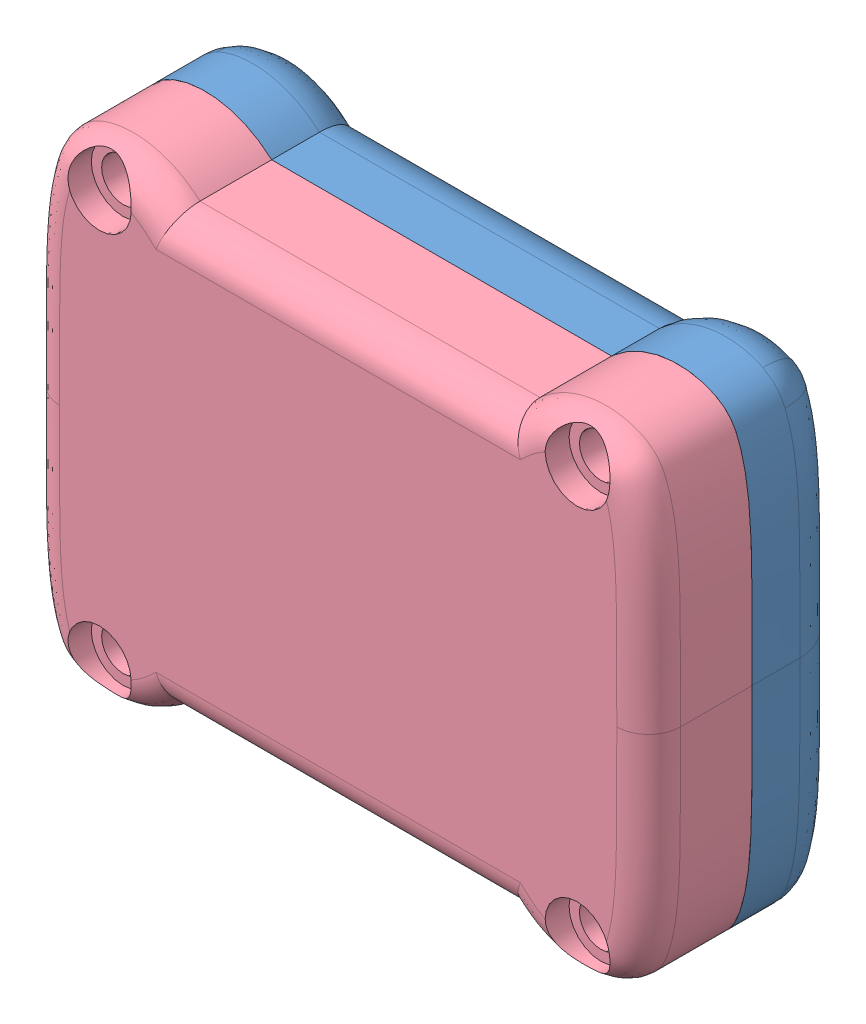
SolidWorks assembly Assem, configuration Default. Lengths in mm.
Overall size (42.86 33.41 13.65).
5 component instances, 4 part files, 6 mates.
Components (placement in the parent):
- Cap-1: Cap [Default] at origin size (42.86 31.57 6.18)
- btn-1: btn [Default] at (-14.2415 0.4663 -1) size (5.36 14.72 4.01)
- Wheel.step-1: Wheel.step [Default] at (16.1914 10.2078 5.1914) size (34.22 20.68 7.76)
- btn-2: btn [Default] at (14.1743 -0.4656 -1) x (-1 0 0) z (0 0 1) size (5.36 14.72 4.01)
- back-1: back [Default] at (-5.148 -1.492 6) size (42.23 33.41 6.65)
Mates (geometry in assembly coordinates):
- Distance1: distance = 2.6 mm anti-aligned: plane of Cap-1 through (0 0 2) normal (0 0 1); plane of Wheel.step-1 through (-13.3336 -10.2672 4.6) normal (0 0 -1)
- Parallel2: parallel anti-aligned: plane of Cap-1 through (-18.9842 11.7725 0) normal (0 0 -1); plane of btn-2 through (15.1399 -4.063 3) normal (0 0 1)
- Coincident4: coincident anti-aligned: plane of Cap-1 through (0 0 2) normal (0 0 1); plane of btn-2 through (15.1399 -4.063 2) normal (0 0 -1)
- Coincident5: coincident anti-aligned: plane of Cap-1 through (-18.9842 11.7725 6) normal (0 0 1); plane of back-1 through (-18.9842 11.7725 6) normal (0 0 -1)
- Concentric1: concentric aligned: circle of Cap-1; circle of back-1
- Coincident7: coincident aligned: plane of btn-1 through (-15.207 4.0637 2) normal (0 0 -1); plane of btn-2 through (15.1399 -4.063 2) normal (0 0 -1)
